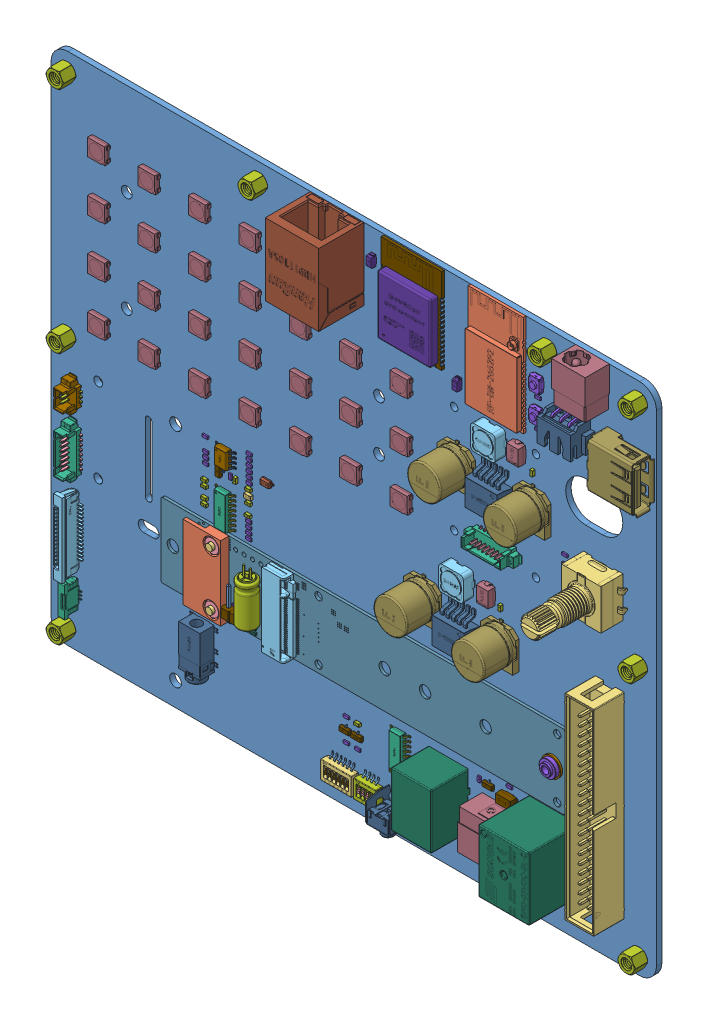
SolidWorks assembly HOUZZkitF1_Tester, configuration 默认. Lengths in mm.
Overall size (180.06 153.05 26.45).
872 component instances, 119 part files, 0 mates.
Components (placement in the parent):
- HOUZZkitF1_Tester.step-1: HOUZZkitF1_Tester.step [默认] at origin size (180.06 153.05 26.45)
  - Board.step-1: Board.step [默认] at origin size (180 153 1.6)
    - Open CASCADE STEP translator 7.5 6.1.1.step-1: Open CASCADE STEP translator 7.5 6.1.1.step [默认] at (0 0 -1.6) size (180 153 1.6)
  - JP4.step-1: JP4.step [默认] at origin size (8.85 58.42 12.17)
    - IDC2.54-40P.step-1: IDC2.54-40P.step [默认] at (77.5 -22.5 0) x (0 1 0) z (0 0 1) size (58.42 8.85 12.17)
      - LOGO__.step-1: LOGO__.step [默认] at (-1.2291 1.1 0.166) x (-1 0 0) z (0 0 -1) size (1.2 1.38 0.01)
      - IDC2.54-40P-0.step-1: IDC2.54-40P-0.step [默认] at origin size (58.42 8.85 12.17)
  - L1.step-1: L1.step [默认] at origin size (7.3 7.3 3.65)
    - CDRH73.step-1: CDRH73.step [默认] at (32.5 36.5 -0.15) x (-1 0 0) z (0 0 1) size (7.3 7.3 3.65)
      - LOGO__-1.step-1: LOGO__-1.step [默认] at (0 0.0189 0.4972) x (-1 0 0) z (0 0 -1) size (0.84 0.97 0.01)
      - CDRH73-2.step-1: CDRH73-2.step [默认] at origin size (7.3 7.3 3.65)
  - C28.step-1: C28.step [默认] at origin size (1.6 0.82 0.82)
    - C 0603.step-1: C 0603.step [默认] at (71 35 -1.6) x (1 0 0) z (0 0 -1) size (1.6 0.82 0.82)
      - LOGO__-3.step-1: LOGO__-3.step [默认] at (0 0.0171 -0.0006) x (-1 0 0) z (0 0 -1) size (0.51 0.59 0)
      - C 0603-4.step-1: C 0603-4.step [默认] at origin size (1.6 0.82 0.82)
  - C26.step-1: C26.step [默认] at origin size (1.6 0.82 0.82)
    - C 0603.step-1: C 0603.step [默认] at (71 16 -1.6) x (1 0 0) z (0 0 -1) size (1.6 0.82 0.82)
      - LOGO__-3.step-1: LOGO__-3.step [默认] at (0 0.0171 -0.0006) x (-1 0 0) z (0 0 -1) size (0.51 0.59 0)
      - C 0603-4.step-1: C 0603-4.step [默认] at origin size (1.6 0.82 0.82)
  - R1.step-1: R1.step [默认] at origin size (1.6 0.8 0.4)
    - R 0603.step-1: R 0603.step [默认] at (63.0001 57.5 0) x (1 0 0) z (0 0 1) size (1.6 0.8 0.4)
      - R 0603-5.step-1: R 0603-5.step [默认] at origin size (1.6 0.8 0.4)
      - LOGO__-6.step-1: LOGO__-6.step [默认] at (0.0001 0.0322 -0.0016) x (-1 0 0) z (0 0 -1) size (0.48 0.55 0)
  - L3.step-1: L3.step [默认] at origin size (7.3 7.3 3.65)
    - CDRH73.step-1: CDRH73.step [默认] at (42 77.5 -0.15) x (-1 0 0) z (0 0 1) size (7.3 7.3 3.65)
      - LOGO__-1.step-1: LOGO__-1.step [默认] at (0 0.0189 0.4972) x (-1 0 0) z (0 0 -1) size (0.84 0.97 0.01)
      - CDRH73-2.step-1: CDRH73-2.step [默认] at origin size (7.3 7.3 3.65)
  - IC5.step-1: IC5.step [默认] at origin size (10 13.33 4.5)
    - TO263-5A.step-1: TO263-5A.step [默认] at (32.5 30 0) x (-1 0 0) z (0 0 1) size (10 13.33 4.5)
  - IC4.step-1: IC4.step [默认] at origin size (10 13.33 4.5)
    - TO263-5A.step-1: TO263-5A.step [默认] at (42.3 70.5 0) x (-1 0 0) z (0 0 1) size (10 13.33 4.5)
  - E7.step-1: E7.step [默认] at origin size (10.3 11.6 10.21)
    - CM F(10X10.2).step-1: CM F(10X10.2).step [默认] at (31 65 0) x (1 0 0) z (0 0 1) size (10.3 11.6 10.21)
      - LOGO__-7.step-1: LOGO__-7.step [默认] at (-0.0044 0.0128 -0.0035) x (-1 0 0) z (0 0 -1) size (1.8 2.08 0.01)
      - CM F(10X10.2)-8.step-1: CM F(10X10.2)-8.step [默认] at origin size (10.3 11.6 10.21)
  - E6.step-1: E6.step [默认] at origin size (10.3 11.6 10.21)
    - CM F(10X10.2).step-1: CM F(10X10.2).step [默认] at (53.5 65 0) x (1 0 0) z (0 0 1) size (10.3 11.6 10.21)
      - LOGO__-7.step-1: LOGO__-7.step [默认] at (-0.0044 0.0128 -0.0035) x (-1 0 0) z (0 0 -1) size (1.8 2.08 0.01)
      - CM F(10X10.2)-8.step-1: CM F(10X10.2)-8.step [默认] at origin size (10.3 11.6 10.21)
  - E5.step-1: E5.step [默认] at origin size (10.3 11.6 10.21)
    - CM F(10X10.2).step-1: CM F(10X10.2).step [默认] at (21 25.5 0) x (1 0 0) z (0 0 1) size (10.3 11.6 10.21)
      - LOGO__-7.step-1: LOGO__-7.step [默认] at (-0.0044 0.0128 -0.0035) x (-1 0 0) z (0 0 -1) size (1.8 2.08 0.01)
      - CM F(10X10.2)-8.step-1: CM F(10X10.2)-8.step [默认] at origin size (10.3 11.6 10.21)
  - E4.step-1: E4.step [默认] at origin size (10.3 11.6 10.21)
    - CM F(10X10.2).step-1: CM F(10X10.2).step [默认] at (44 25.5 0) x (1 0 0) z (0 0 1) size (10.3 11.6 10.21)
      - LOGO__-7.step-1: LOGO__-7.step [默认] at (-0.0044 0.0128 -0.0035) x (-1 0 0) z (0 0 -1) size (1.8 2.08 0.01)
      - CM F(10X10.2)-8.step-1: CM F(10X10.2)-8.step [默认] at origin size (10.3 11.6 10.21)
  - D4.step-1: D4.step [默认] at origin size (3.6 5.31 2.31)
    - SMB.step-1: SMB.step [默认] at (49.5001 77.4771 0.05) x (0 1 0) z (0 0 1) size (5.31 3.6 2.31)
      - SMB-9.step-1: SMB-9.step [默认] at origin size (5.31 3.6 2.3)
      - LOGO__________.____.step-1: LOGO__________.____.step [默认] at (-0.0044 0 -0.003) x (-1 0 0) z (0 0 -1) size (0.9 1.04 0.01)
  - D3.step-1: D3.step [默认] at origin size (3.6 5.31 2.31)
    - SMB.step-1: SMB.step [默认] at (40.5001 36.4771 0.05) x (0 1 0) z (0 0 1) size (5.31 3.6 2.31)
      - SMB-9.step-1: SMB-9.step [默认] at origin size (5.31 3.6 2.3)
      - LOGO__________.____.step-1: LOGO__________.____.step [默认] at (-0.0044 0 -0.003) x (-1 0 0) z (0 0 -1) size (0.9 1.04 0.01)
  - U7.step-1: U7.step [默认] at origin size (10.31 17.9 2.7)
    - SOP28.step-1: SOP28.step [默认] at (62.5 32.5 -1.6) x (1 0 0) z (0 0 -1) size (10.31 17.9 2.7)
      - LOGO__0.5.step-1: LOGO__0.5.step [默认] at (0.0116 0 0.095) x (0 -1 0) z (0 0 -1) size (1.5 1.73 0.01)
      - SOP28 ____.step-1: SOP28 ____.step [默认] at origin size (7.7 17.9 2.6)
      - ________2.6 ____________.step-1: ________2.6 ____________.step [默认] at (3.85 8.26 1.4) x (0 1 0) z (0 0 1) size (0.5 1.3 1.5)
      - ________2.6 ____________.step-2: ________2.6 ____________.step [默认] at (3.85 6.99 1.4) x (0 1 0) z (0 0 1) size (0.5 1.3 1.5)
      - ________2.6 ____________.step-3: ________2.6 ____________.step [默认] at (3.85 5.72 1.4) x (0 1 0) z (0 0 1) size (0.5 1.3 1.5)
      - ________2.6 ____________.step-4: ________2.6 ____________.step [默认] at (3.85 4.45 1.4) x (0 1 0) z (0 0 1) size (0.5 1.3 1.5)
      - ________2.6 ____________.step-5: ________2.6 ____________.step [默认] at (3.85 3.18 1.4) x (0 1 0) z (0 0 1) size (0.5 1.3 1.5)
      - ________2.6 ____________.step-6: ________2.6 ____________.step [默认] at (3.85 1.91 1.4) x (0 1 0) z (0 0 1) size (0.5 1.3 1.5)
      - ________2.6 ____________.step-7: ________2.6 ____________.step [默认] at (3.85 0.64 1.4) x (0 1 0) z (0 0 1) size (0.5 1.3 1.5)
      - ________2.6 ____________.step-8: ________2.6 ____________.step [默认] at (3.85 -0.63 1.4) x (0 1 0) z (0 0 1) size (0.5 1.3 1.5)
      - ________2.6 ____________.step-9: ________2.6 ____________.step [默认] at (3.85 -1.9 1.4) x (0 1 0) z (0 0 1) size (0.5 1.3 1.5)
      - ________2.6 ____________.step-10: ________2.6 ____________.step [默认] at (3.85 -3.17 1.4) x (0 1 0) z (0 0 1) size (0.5 1.3 1.5)
      - ________2.6 ____________.step-11: ________2.6 ____________.step [默认] at (3.85 -4.44 1.4) x (0 1 0) z (0 0 1) size (0.5 1.3 1.5)
      - ________2.6 ____________.step-12: ________2.6 ____________.step [默认] at (3.85 -5.71 1.4) x (0 1 0) z (0 0 1) size (0.5 1.3 1.5)
      - ________2.6 ____________.step-13: ________2.6 ____________.step [默认] at (3.85 -6.98 1.4) x (0 1 0) z (0 0 1) size (0.5 1.3 1.5)
      - ________2.6 ____________.step-14: ________2.6 ____________.step [默认] at (3.85 -8.25 1.4) x (0 1 0) z (0 0 1) size (0.5 1.3 1.5)
      - ________2.6 ____________.step-15: ________2.6 ____________.step [默认] at (-3.85 8.26 1.4) x (0 -1 0) z (0 0 1) size (0.5 1.3 1.5)
      - ________2.6 ____________.step-16: ________2.6 ____________.step [默认] at (-3.85 6.99 1.4) x (0 -1 0) z (0 0 1) size (0.5 1.3 1.5)
      - ________2.6 ____________.step-17: ________2.6 ____________.step [默认] at (-3.85 5.72 1.4) x (0 -1 0) z (0 0 1) size (0.5 1.3 1.5)
      - ________2.6 ____________.step-18: ________2.6 ____________.step [默认] at (-3.85 4.45 1.4) x (0 -1 0) z (0 0 1) size (0.5 1.3 1.5)
      - ________2.6 ____________.step-19: ________2.6 ____________.step [默认] at (-3.85 3.18 1.4) x (0 -1 0) z (0 0 1) size (0.5 1.3 1.5)
      - ________2.6 ____________.step-20: ________2.6 ____________.step [默认] at (-3.85 1.91 1.4) x (0 -1 0) z (0 0 1) size (0.5 1.3 1.5)
      - ________2.6 ____________.step-21: ________2.6 ____________.step [默认] at (-3.85 0.64 1.4) x (0 -1 0) z (0 0 1) size (0.5 1.3 1.5)
      - ________2.6 ____________.step-22: ________2.6 ____________.step [默认] at (-3.85 -0.63 1.4) x (0 -1 0) z (0 0 1) size (0.5 1.3 1.5)
      - ________2.6 ____________.step-23: ________2.6 ____________.step [默认] at (-3.85 -1.9 1.4) x (0 -1 0) z (0 0 1) size (0.5 1.3 1.5)
      - ________2.6 ____________.step-24: ________2.6 ____________.step [默认] at (-3.85 -3.17 1.4) x (0 -1 0) z (0 0 1) size (0.5 1.3 1.5)
      - ________2.6 ____________.step-25: ________2.6 ____________.step [默认] at (-3.85 -4.44 1.4) x (0 -1 0) z (0 0 1) size (0.5 1.3 1.5)
      - ________2.6 ____________.step-26: ________2.6 ____________.step [默认] at (-3.85 -5.71 1.4) x (0 -1 0) z (0 0 1) size (0.5 1.3 1.5)
      - ________2.6 ____________.step-27: ________2.6 ____________.step [默认] at (-3.85 -6.98 1.4) x (0 -1 0) z (0 0 1) size (0.5 1.3 1.5)
      - ________2.6 ____________.step-28: ________2.6 ____________.step [默认] at (-3.85 -8.25 1.4) x (0 -1 0) z (0 0 1) size (0.5 1.3 1.5)
  - U6.step-1: U6.step [默认] at origin size (10.31 17.9 2.7)
    - SOP28.step-1: SOP28.step [默认] at (62.5 13.5 -1.6) x (1 0 0) z (0 0 -1) size (10.31 17.9 2.7)
      - LOGO__0.5.step-1: LOGO__0.5.step [默认] at (0.0116 0 0.095) x (0 -1 0) z (0 0 -1) size (1.5 1.73 0.01)
      - SOP28 ____.step-1: SOP28 ____.step [默认] at origin size (7.7 17.9 2.6)
      - ________2.6 ____________.step-1: ________2.6 ____________.step [默认] at (3.85 8.26 1.4) x (0 1 0) z (0 0 1) size (0.5 1.3 1.5)
      - ________2.6 ____________.step-2: ________2.6 ____________.step [默认] at (3.85 6.99 1.4) x (0 1 0) z (0 0 1) size (0.5 1.3 1.5)
      - ________2.6 ____________.step-3: ________2.6 ____________.step [默认] at (3.85 5.72 1.4) x (0 1 0) z (0 0 1) size (0.5 1.3 1.5)
      - ________2.6 ____________.step-4: ________2.6 ____________.step [默认] at (3.85 4.45 1.4) x (0 1 0) z (0 0 1) size (0.5 1.3 1.5)
      - ________2.6 ____________.step-5: ________2.6 ____________.step [默认] at (3.85 3.18 1.4) x (0 1 0) z (0 0 1) size (0.5 1.3 1.5)
      - ________2.6 ____________.step-6: ________2.6 ____________.step [默认] at (3.85 1.91 1.4) x (0 1 0) z (0 0 1) size (0.5 1.3 1.5)
      - ________2.6 ____________.step-7: ________2.6 ____________.step [默认] at (3.85 0.64 1.4) x (0 1 0) z (0 0 1) size (0.5 1.3 1.5)
      - ________2.6 ____________.step-8: ________2.6 ____________.step [默认] at (3.85 -0.63 1.4) x (0 1 0) z (0 0 1) size (0.5 1.3 1.5)
      - ________2.6 ____________.step-9: ________2.6 ____________.step [默认] at (3.85 -1.9 1.4) x (0 1 0) z (0 0 1) size (0.5 1.3 1.5)
      - ________2.6 ____________.step-10: ________2.6 ____________.step [默认] at (3.85 -3.17 1.4) x (0 1 0) z (0 0 1) size (0.5 1.3 1.5)
      - ________2.6 ____________.step-11: ________2.6 ____________.step [默认] at (3.85 -4.44 1.4) x (0 1 0) z (0 0 1) size (0.5 1.3 1.5)
      - ________2.6 ____________.step-12: ________2.6 ____________.step [默认] at (3.85 -5.71 1.4) x (0 1 0) z (0 0 1) size (0.5 1.3 1.5)
      - ________2.6 ____________.step-13: ________2.6 ____________.step [默认] at (3.85 -6.98 1.4) x (0 1 0) z (0 0 1) size (0.5 1.3 1.5)
      - ________2.6 ____________.step-14: ________2.6 ____________.step [默认] at (3.85 -8.25 1.4) x (0 1 0) z (0 0 1) size (0.5 1.3 1.5)
      - ________2.6 ____________.step-15: ________2.6 ____________.step [默认] at (-3.85 8.26 1.4) x (0 -1 0) z (0 0 1) size (0.5 1.3 1.5)
      - ________2.6 ____________.step-16: ________2.6 ____________.step [默认] at (-3.85 6.99 1.4) x (0 -1 0) z (0 0 1) size (0.5 1.3 1.5)
      - ________2.6 ____________.step-17: ________2.6 ____________.step [默认] at (-3.85 5.72 1.4) x (0 -1 0) z (0 0 1) size (0.5 1.3 1.5)
      - ________2.6 ____________.step-18: ________2.6 ____________.step [默认] at (-3.85 4.45 1.4) x (0 -1 0) z (0 0 1) size (0.5 1.3 1.5)
      - ________2.6 ____________.step-19: ________2.6 ____________.step [默认] at (-3.85 3.18 1.4) x (0 -1 0) z (0 0 1) size (0.5 1.3 1.5)
      - ________2.6 ____________.step-20: ________2.6 ____________.step [默认] at (-3.85 1.91 1.4) x (0 -1 0) z (0 0 1) size (0.5 1.3 1.5)
      - ________2.6 ____________.step-21: ________2.6 ____________.step [默认] at (-3.85 0.64 1.4) x (0 -1 0) z (0 0 1) size (0.5 1.3 1.5)
      - ________2.6 ____________.step-22: ________2.6 ____________.step [默认] at (-3.85 -0.63 1.4) x (0 -1 0) z (0 0 1) size (0.5 1.3 1.5)
      - ________2.6 ____________.step-23: ________2.6 ____________.step [默认] at (-3.85 -1.9 1.4) x (0 -1 0) z (0 0 1) size (0.5 1.3 1.5)
      - ________2.6 ____________.step-24: ________2.6 ____________.step [默认] at (-3.85 -3.17 1.4) x (0 -1 0) z (0 0 1) size (0.5 1.3 1.5)
      - ________2.6 ____________.step-25: ________2.6 ____________.step [默认] at (-3.85 -4.44 1.4) x (0 -1 0) z (0 0 1) size (0.5 1.3 1.5)
      - ________2.6 ____________.step-26: ________2.6 ____________.step [默认] at (-3.85 -5.71 1.4) x (0 -1 0) z (0 0 1) size (0.5 1.3 1.5)
      - ________2.6 ____________.step-27: ________2.6 ____________.step [默认] at (-3.85 -6.98 1.4) x (0 -1 0) z (0 0 1) size (0.5 1.3 1.5)
      - ________2.6 ____________.step-28: ________2.6 ____________.step [默认] at (-3.85 -8.25 1.4) x (0 -1 0) z (0 0 1) size (0.5 1.3 1.5)
  - R51.step-1: R51.step [默认] at origin size (1.6 0.8 0.4)
    - R 0603.step-1: R 0603.step [默认] at (71.0001 36.5 -1.6) x (1 0 0) z (0 0 -1) size (1.6 0.8 0.4)
      - R 0603-5.step-1: R 0603-5.step [默认] at origin size (1.6 0.8 0.4)
      - LOGO__-6.step-1: LOGO__-6.step [默认] at (0.0001 0.0322 -0.0016) x (-1 0 0) z (0 0 -1) size (0.48 0.55 0)
  - R50.step-1: R50.step [默认] at origin size (1.6 0.8 0.4)
    - R 0603.step-1: R 0603.step [默认] at (71.0001 38 -1.6) x (1 0 0) z (0 0 -1) size (1.6 0.8 0.4)
      - R 0603-5.step-1: R 0603-5.step [默认] at origin size (1.6 0.8 0.4)
      - LOGO__-6.step-1: LOGO__-6.step [默认] at (0.0001 0.0322 -0.0016) x (-1 0 0) z (0 0 -1) size (0.48 0.55 0)
  - R49.step-1: R49.step [默认] at origin size (1.6 0.8 0.4)
    - R 0603.step-1: R 0603.step [默认] at (71.0001 39.5 -1.6) x (1 0 0) z (0 0 -1) size (1.6 0.8 0.4)
      - R 0603-5.step-1: R 0603-5.step [默认] at origin size (1.6 0.8 0.4)
      - LOGO__-6.step-1: LOGO__-6.step [默认] at (0.0001 0.0322 -0.0016) x (-1 0 0) z (0 0 -1) size (0.48 0.55 0)
  - R48.step-1: R48.step [默认] at origin size (1.6 0.8 0.4)
    - R 0603.step-1: R 0603.step [默认] at (54.0001 39 -1.6) x (1 0 0) z (0 0 -1) size (1.6 0.8 0.4)
      - R 0603-5.step-1: R 0603-5.step [默认] at origin size (1.6 0.8 0.4)
      - LOGO__-6.step-1: LOGO__-6.step [默认] at (0.0001 0.0322 -0.0016) x (-1 0 0) z (0 0 -1) size (0.48 0.55 0)
  - R47.step-1: R47.step [默认] at origin size (1.6 0.8 0.4)
    - R 0603.step-1: R 0603.step [默认] at (71.0001 17.5 -1.6) x (1 0 0) z (0 0 -1) size (1.6 0.8 0.4)
      - R 0603-5.step-1: R 0603-5.step [默认] at origin size (1.6 0.8 0.4)
      - LOGO__-6.step-1: LOGO__-6.step [默认] at (0.0001 0.0322 -0.0016) x (-1 0 0) z (0 0 -1) size (0.48 0.55 0)
  - R46.step-1: R46.step [默认] at origin size (1.6 0.8 0.4)
    - R 0603.step-1: R 0603.step [默认] at (71.0001 19 -1.6) x (1 0 0) z (0 0 -1) size (1.6 0.8 0.4)
      - R 0603-5.step-1: R 0603-5.step [默认] at origin size (1.6 0.8 0.4)
      - LOGO__-6.step-1: LOGO__-6.step [默认] at (0.0001 0.0322 -0.0016) x (-1 0 0) z (0 0 -1) size (0.48 0.55 0)
  - R45.step-1: R45.step [默认] at origin size (1.6 0.8 0.4)
    - R 0603.step-1: R 0603.step [默认] at (71.0001 20.5 -1.6) x (1 0 0) z (0 0 -1) size (1.6 0.8 0.4)
      - R 0603-5.step-1: R 0603-5.step [默认] at origin size (1.6 0.8 0.4)
      - LOGO__-6.step-1: LOGO__-6.step [默认] at (0.0001 0.0322 -0.0016) x (-1 0 0) z (0 0 -1) size (0.48 0.55 0)
  - R44.step-1: R44.step [默认] at origin size (1.6 0.8 0.4)
    - R 0603.step-1: R 0603.step [默认] at (54.0001 16.4999 -1.6) x (1 0 0) z (0 0 -1) size (1.6 0.8 0.4)
      - R 0603-5.step-1: R 0603-5.step [默认] at origin size (1.6 0.8 0.4)
      - LOGO__-6.step-1: LOGO__-6.step [默认] at (0.0001 0.0322 -0.0016) x (-1 0 0) z (0 0 -1) size (0.48 0.55 0)
  - R43.step-1: R43.step [默认] at origin size (1.6 0.8 0.4)
    - R 0603.step-1: R 0603.step [默认] at (-31.0001 14.5999 0) x (-1 0 0) z (0 0 1) size (1.6 0.8 0.4)
      - R 0603-5.step-1: R 0603-5.step [默认] at origin size (1.6 0.8 0.4)
      - LOGO__-6.step-1: LOGO__-6.step [默认] at (0.0001 0.0322 -0.0016) x (-1 0 0) z (0 0 -1) size (0.48 0.55 0)
  - R42.step-1: R42.step [默认] at origin size (1.6 0.8 0.4)
    - R 0603.step-1: R 0603.step [默认] at (-31.0001 16.0999 0) x (-1 0 0) z (0 0 1) size (1.6 0.8 0.4)
      - R 0603-5.step-1: R 0603-5.step [默认] at origin size (1.6 0.8 0.4)
      - LOGO__-6.step-1: LOGO__-6.step [默认] at (0.0001 0.0322 -0.0016) x (-1 0 0) z (0 0 -1) size (0.48 0.55 0)
  - R41.step-1: R41.step [默认] at origin size (1.6 0.8 0.4)
    - R 0603.step-1: R 0603.step [默认] at (-31.0001 17.5999 0) x (-1 0 0) z (0 0 1) size (1.6 0.8 0.4)
      - R 0603-5.step-1: R 0603-5.step [默认] at origin size (1.6 0.8 0.4)
      - LOGO__-6.step-1: LOGO__-6.step [默认] at (0.0001 0.0322 -0.0016) x (-1 0 0) z (0 0 -1) size (0.48 0.55 0)
  - R40.step-1: R40.step [默认] at origin size (1.6 0.8 0.4)
    - R 0603.step-1: R 0603.step [默认] at (-31.0001 19.0999 0) x (-1 0 0) z (0 0 1) size (1.6 0.8 0.4)
      - R 0603-5.step-1: R 0603-5.step [默认] at origin size (1.6 0.8 0.4)
      - LOGO__-6.step-1: LOGO__-6.step [默认] at (0.0001 0.0322 -0.0016) x (-1 0 0) z (0 0 -1) size (0.48 0.55 0)
  - R39.step-1: R39.step [默认] at origin size (1.6 0.8 0.4)
    - R 0603.step-1: R 0603.step [默认] at (-43.7999 27.6 0) x (1 0 0) z (0 0 1) size (1.6 0.8 0.4)
      - R 0603-5.step-1: R 0603-5.step [默认] at origin size (1.6 0.8 0.4)
      - LOGO__-6.step-1: LOGO__-6.step [默认] at (0.0001 0.0322 -0.0016) x (-1 0 0) z (0 0 -1) size (0.48 0.55 0)
  - R38.step-1: R38.step [默认] at origin size (1.6 0.8 0.4)
    - R 0603.step-1: R 0603.step [默认] at (-30.9001 33.5 0) x (-1 0 0) z (0 0 1) size (1.6 0.8 0.4)
      - R 0603-5.step-1: R 0603-5.step [默认] at origin size (1.6 0.8 0.4)
      - LOGO__-6.step-1: LOGO__-6.step [默认] at (0.0001 0.0322 -0.0016) x (-1 0 0) z (0 0 -1) size (0.48 0.55 0)
  - R37.step-1: R37.step [默认] at origin size (1.6 0.8 0.4)
    - R 0603.step-1: R 0603.step [默认] at (-43.8001 29.0999 0) x (-1 0 0) z (0 0 1) size (1.6 0.8 0.4)
      - R 0603-5.step-1: R 0603-5.step [默认] at origin size (1.6 0.8 0.4)
      - LOGO__-6.step-1: LOGO__-6.step [默认] at (0.0001 0.0322 -0.0016) x (-1 0 0) z (0 0 -1) size (0.48 0.55 0)
  - R36.step-1: R36.step [默认] at origin size (1.6 0.8 0.4)
    - R 0603.step-1: R 0603.step [默认] at (-43.8001 30.5999 0) x (-1 0 0) z (0 0 1) size (1.6 0.8 0.4)
      - R 0603-5.step-1: R 0603-5.step [默认] at origin size (1.6 0.8 0.4)
      - LOGO__-6.step-1: LOGO__-6.step [默认] at (0.0001 0.0322 -0.0016) x (-1 0 0) z (0 0 -1) size (0.48 0.55 0)
  - R35.step-1: R35.step [默认] at origin size (1.6 0.8 0.4)
    - R 0603.step-1: R 0603.step [默认] at (-30.9001 30.5 0) x (-1 0 0) z (0 0 1) size (1.6 0.8 0.4)
      - R 0603-5.step-1: R 0603-5.step [默认] at origin size (1.6 0.8 0.4)
      - LOGO__-6.step-1: LOGO__-6.step [默认] at (0.0001 0.0322 -0.0016) x (-1 0 0) z (0 0 -1) size (0.48 0.55 0)
  - R34.step-1: R34.step [默认] at origin size (1.6 0.8 0.4)
    - R 0603.step-1: R 0603.step [默认] at (-30.9001 35 0) x (-1 0 0) z (0 0 1) size (1.6 0.8 0.4)
      - R 0603-5.step-1: R 0603-5.step [默认] at origin size (1.6 0.8 0.4)
      - LOGO__-6.step-1: LOGO__-6.step [默认] at (0.0001 0.0322 -0.0016) x (-1 0 0) z (0 0 -1) size (0.48 0.55 0)
  - R33.step-1: R33.step [默认] at origin size (1.6 0.8 0.4)
    - R 0603.step-1: R 0603.step [默认] at (-43.8999 34.5001 0) x (1 0 0) z (0 0 1) size (1.6 0.8 0.4)
      - R 0603-5.step-1: R 0603-5.step [默认] at origin size (1.6 0.8 0.4)
      - LOGO__-6.step-1: LOGO__-6.step [默认] at (0.0001 0.0322 -0.0016) x (-1 0 0) z (0 0 -1) size (0.48 0.55 0)
  - R32.step-1: R32.step [默认] at origin size (1.6 0.8 0.4)
    - R 0603.step-1: R 0603.step [默认] at (-30.8999 32.0001 0) x (1 0 0) z (0 0 1) size (1.6 0.8 0.4)
      - R 0603-5.step-1: R 0603-5.step [默认] at origin size (1.6 0.8 0.4)
      - LOGO__-6.step-1: LOGO__-6.step [默认] at (0.0001 0.0322 -0.0016) x (-1 0 0) z (0 0 -1) size (0.48 0.55 0)
  - R31.step-1: R31.step [默认] at origin size (1.6 0.8 0.4)
    - R 0603.step-1: R 0603.step [默认] at (-30.9001 29 0) x (-1 0 0) z (0 0 1) size (1.6 0.8 0.4)
      - R 0603-5.step-1: R 0603-5.step [默认] at origin size (1.6 0.8 0.4)
      - LOGO__-6.step-1: LOGO__-6.step [默认] at (0.0001 0.0322 -0.0016) x (-1 0 0) z (0 0 -1) size (0.48 0.55 0)
  - R30.step-1: R30.step [默认] at origin size (0.8 1.6 0.4)
    - R 0603.step-1: R 0603.step [默认] at (-36.5 27.9001 0) x (0 1 0) z (0 0 1) size (1.6 0.8 0.4)
      - R 0603-5.step-1: R 0603-5.step [默认] at origin size (1.6 0.8 0.4)
      - LOGO__-6.step-1: LOGO__-6.step [默认] at (0.0001 0.0322 -0.0016) x (-1 0 0) z (0 0 -1) size (0.48 0.55 0)
  - R29.step-1: R29.step [默认] at origin size (1.6 0.8 0.4)
    - R 0603.step-1: R 0603.step [默认] at (-30.9001 36.5 0) x (-1 0 0) z (0 0 1) size (1.6 0.8 0.4)
      - R 0603-5.step-1: R 0603-5.step [默认] at origin size (1.6 0.8 0.4)
      - LOGO__-6.step-1: LOGO__-6.step [默认] at (0.0001 0.0322 -0.0016) x (-1 0 0) z (0 0 -1) size (0.48 0.55 0)
  - Q4.step-1: Q4.step [默认] at origin size (2.4 3 1.05)
    - SOT23-3.step-1: SOT23-3.step [默认] at (-39.6 28 0) x (0 -1 0) z (0 0 1) size (3 2.4 1.05)
      - SOT23-3-10.step-1: SOT23-3-10.step [默认] at origin size (3 1.3 1)
      - SOT23-3 ______.step-1: SOT23-3 ______.step [默认] at (0 0.5461 0.475) size (0.4 0.65 0.55)
      - SOT23-3 ______.step-2: SOT23-3 ______.step [默认] at (-0.95 -0.5461 0.475) x (-1 0 0) z (0 0 1) size (0.4 0.65 0.55)
      - SOT23-3 ______.step-3: SOT23-3 ______.step [默认] at (0.95 -0.5461 0.475) x (-1 0 0) z (0 0 1) size (0.4 0.65 0.55)
      - LOGO__0.15.step-1: LOGO__0.15.step [默认] at (0 -0.0163 0.0485) x (-1 0 0) z (0 0 -1) size (0.45 0.52 0)
  - LB2.step-1: LB2.step [默认] at origin size (2.01 1.21 0.91)
    - FB 0805.step-1: FB 0805.step [默认] at (-30.9 25.7 0) x (-1 0 0) z (0 1 0) size (2 0.91 1.2)
      - FB 0805-11.step-1: FB 0805-11.step [默认] at origin size (2 0.91 1.2)
      - LOGO__0.15-12.step-1: LOGO__0.15-12.step [默认] at (-0.0107 -0.0015 -0.0162) x (1 0 0) z (0 1 0) size (0.45 0.52 0)
  - IC3.step-1: IC3.step [默认] at origin size (6.01 10 1.9)
    - SOP16.step-1: SOP16.step [默认] at (-38 19 0) x (1 0 0) z (0 0 1) size (6.01 10 1.9)
      - LOGO__0.25.step-1: LOGO__0.25.step [默认] at (0.0116 0 0.095) x (0 -1 0) z (0 0 -1) size (0.75 0.87 0.01)
      - SOP16 ____.step-1: SOP16 ____.step [默认] at origin size (3.6 10 1.8)
      - ________1.8 ____________.step-1: ________1.8 ____________.step [默认] at (1.8 4.45 1) x (0 1 0) z (0 0 1) size (0.5 1.2 1.1)
      - ________1.8 ____________.step-2: ________1.8 ____________.step [默认] at (1.8 3.18 1) x (0 1 0) z (0 0 1) size (0.5 1.2 1.1)
      - ________1.8 ____________.step-3: ________1.8 ____________.step [默认] at (1.8 1.91 1) x (0 1 0) z (0 0 1) size (0.5 1.2 1.1)
      - ________1.8 ____________.step-4: ________1.8 ____________.step [默认] at (1.8 0.64 1) x (0 1 0) z (0 0 1) size (0.5 1.2 1.1)
      - ________1.8 ____________.step-5: ________1.8 ____________.step [默认] at (1.8 -0.63 1) x (0 1 0) z (0 0 1) size (0.5 1.2 1.1)
      - ________1.8 ____________.step-6: ________1.8 ____________.step [默认] at (1.8 -1.9 1) x (0 1 0) z (0 0 1) size (0.5 1.2 1.1)
      - ________1.8 ____________.step-7: ________1.8 ____________.step [默认] at (1.8 -3.17 1) x (0 1 0) z (0 0 1) size (0.5 1.2 1.1)
      - ________1.8 ____________.step-8: ________1.8 ____________.step [默认] at (1.8 -4.44 1) x (0 1 0) z (0 0 1) size (0.5 1.2 1.1)
      - ________1.8 ____________.step-9: ________1.8 ____________.step [默认] at (-1.8 4.45 1) x (0 -1 0) z (0 0 1) size (0.5 1.2 1.1)
      - ________1.8 ____________.step-10: ________1.8 ____________.step [默认] at (-1.8 3.18 1) x (0 -1 0) z (0 0 1) size (0.5 1.2 1.1)
      - ________1.8 ____________.step-11: ________1.8 ____________.step [默认] at (-1.8 1.91 1) x (0 -1 0) z (0 0 1) size (0.5 1.2 1.1)
      - ________1.8 ____________.step-12: ________1.8 ____________.step [默认] at (-1.8 0.64 1) x (0 -1 0) z (0 0 1) size (0.5 1.2 1.1)
      - ________1.8 ____________.step-13: ________1.8 ____________.step [默认] at (-1.8 -0.63 1) x (0 -1 0) z (0 0 1) size (0.5 1.2 1.1)
      - ________1.8 ____________.step-14: ________1.8 ____________.step [默认] at (-1.8 -1.9 1) x (0 -1 0) z (0 0 1) size (0.5 1.2 1.1)
      - ________1.8 ____________.step-15: ________1.8 ____________.step [默认] at (-1.8 -3.17 1) x (0 -1 0) z (0 0 1) size (0.5 1.2 1.1)
      - ________1.8 ____________.step-16: ________1.8 ____________.step [默认] at (-1.8 -4.44 1) x (0 -1 0) z (0 0 1) size (0.5 1.2 1.1)
  - IC2.step-1: IC2.step [默认] at origin size (6.01 5 1.9)
    - SOP8.step-1: SOP8.step [默认] at (-37.9 32.6 0) size (6.01 5 1.9)
      - LOGO__0.25-13.step-1: LOGO__0.25-13.step [默认] at (0.0116 0 0.095) x (0 -1 0) z (0 0 -1) size (0.75 0.87 0.01)
      - SOP8 ____.step-1: SOP8 ____.step [默认] at origin size (3.6 5 1.8)
      - ________1.8 ____________-14.step-1: ________1.8 ____________-14.step [默认] at (1.8 1.91 1) x (0 1 0) z (0 0 1) size (0.5 1.2 1.1)
      - ________1.8 ____________-14.step-2: ________1.8 ____________-14.step [默认] at (1.8 0.64 1) x (0 1 0) z (0 0 1) size (0.5 1.2 1.1)
      - ________1.8 ____________-14.step-3: ________1.8 ____________-14.step [默认] at (1.8 -0.63 1) x (0 1 0) z (0 0 1) size (0.5 1.2 1.1)
      - ________1.8 ____________-14.step-4: ________1.8 ____________-14.step [默认] at (1.8 -1.9 1) x (0 1 0) z (0 0 1) size (0.5 1.2 1.1)
      - ________1.8 ____________-14.step-5: ________1.8 ____________-14.step [默认] at (-1.8 1.91 1) x (0 -1 0) z (0 0 1) size (0.5 1.2 1.1)
      - ________1.8 ____________-14.step-6: ________1.8 ____________-14.step [默认] at (-1.8 0.64 1) x (0 -1 0) z (0 0 1) size (0.5 1.2 1.1)
      - ________1.8 ____________-14.step-7: ________1.8 ____________-14.step [默认] at (-1.8 -0.63 1) x (0 -1 0) z (0 0 1) size (0.5 1.2 1.1)
      - ________1.8 ____________-14.step-8: ________1.8 ____________-14.step [默认] at (-1.8 -1.9 1) x (0 -1 0) z (0 0 1) size (0.5 1.2 1.1)
  - D2.step-1: D2.step [默认] at origin size (3.7 1.6 1.22)
    - SOD-123.step-1: SOD-123.step [默认] at (-25.5 32 0.05) x (1 0 0) z (0 0 1) size (3.7 1.6 1.22)
      - SOD-123-15.step-1: SOD-123-15.step [默认] at origin size (3.7 1.6 1.22)
      - LOGO__________.____-16.step-1: LOGO__________.____-16.step [默认] at (-0.0155 0.0364 -0.003) x (-1 0 0) z (0 0 -1) size (0.9 1.04 0.01)
  - C29.step-1: C29.step [默认] at origin size (1.6 0.82 0.82)
    - C 0603.step-1: C 0603.step [默认] at (54 37.5 -1.6) x (1 0 0) z (0 0 -1) size (1.6 0.82 0.82)
      - LOGO__-3.step-1: LOGO__-3.step [默认] at (0 0.0171 -0.0006) x (-1 0 0) z (0 0 -1) size (0.51 0.59 0)
      - C 0603-4.step-1: C 0603-4.step [默认] at origin size (1.6 0.82 0.82)
  - C27.step-1: C27.step [默认] at origin size (1.6 0.82 0.82)
    - C 0603.step-1: C 0603.step [默认] at (54 15 -1.6) x (1 0 0) z (0 0 -1) size (1.6 0.82 0.82)
      - LOGO__-3.step-1: LOGO__-3.step [默认] at (0 0.0171 -0.0006) x (-1 0 0) z (0 0 -1) size (0.51 0.59 0)
      - C 0603-4.step-1: C 0603-4.step [默认] at origin size (1.6 0.82 0.82)
  - C25.step-1: C25.step [默认] at origin size (1.6 0.82 0.82)
    - C 0603.step-1: C 0603.step [默认] at (-44 17.1 0) x (-1 0 0) z (0 0 1) size (1.6 0.82 0.82)
      - LOGO__-3.step-1: LOGO__-3.step [默认] at (0 0.0171 -0.0006) x (-1 0 0) z (0 0 -1) size (0.51 0.59 0)
      - C 0603-4.step-1: C 0603-4.step [默认] at origin size (1.6 0.82 0.82)
  - C24.step-1: C24.step [默认] at origin size (1.6 0.82 0.82)
    - C 0603.step-1: C 0603.step [默认] at (-44 18.7 0) x (-1 0 0) z (0 0 1) size (1.6 0.82 0.82)
      - LOGO__-3.step-1: LOGO__-3.step [默认] at (0 0.0171 -0.0006) x (-1 0 0) z (0 0 -1) size (0.51 0.59 0)
      - C 0603-4.step-1: C 0603-4.step [默认] at origin size (1.6 0.82 0.82)
  - C23.step-1: C23.step [默认] at origin size (1.6 0.82 0.82)
    - C 0603.step-1: C 0603.step [默认] at (-44 23.4 0) x (1 0 0) z (0 0 1) size (1.6 0.82 0.82)
      - LOGO__-3.step-1: LOGO__-3.step [默认] at (0 0.0171 -0.0006) x (-1 0 0) z (0 0 -1) size (0.51 0.59 0)
      - C 0603-4.step-1: C 0603-4.step [默认] at origin size (1.6 0.82 0.82)
  - C22.step-1: C22.step [默认] at origin size (1.6 0.82 0.82)
    - C 0603.step-1: C 0603.step [默认] at (-44 21.8 0) x (-1 0 0) z (0 0 1) size (1.6 0.82 0.82)
      - LOGO__-3.step-1: LOGO__-3.step [默认] at (0 0.0171 -0.0006) x (-1 0 0) z (0 0 -1) size (0.51 0.59 0)
      - C 0603-4.step-1: C 0603-4.step [默认] at origin size (1.6 0.82 0.82)
  - C21.step-1: C21.step [默认] at origin size (1.6 0.82 0.82)
    - C 0603.step-1: C 0603.step [默认] at (-31 20.7 0) x (-1 0 0) z (0 0 1) size (1.6 0.82 0.82)
      - LOGO__-3.step-1: LOGO__-3.step [默认] at (0 0.0171 -0.0006) x (-1 0 0) z (0 0 -1) size (0.51 0.59 0)
      - C 0603-4.step-1: C 0603-4.step [默认] at origin size (1.6 0.82 0.82)
  - C20.step-1: C20.step [默认] at origin size (1.6 0.82 0.82)
    - C 0603.step-1: C 0603.step [默认] at (-30.9 23.9 0) x (-1 0 0) z (0 0 1) size (1.6 0.82 0.82)
      - LOGO__-3.step-1: LOGO__-3.step [默认] at (0 0.0171 -0.0006) x (-1 0 0) z (0 0 -1) size (0.51 0.59 0)
      - C 0603-4.step-1: C 0603-4.step [默认] at origin size (1.6 0.82 0.82)
  - C19.step-1: C19.step [默认] at origin size (1.6 0.82 0.82)
    - C 0603.step-1: C 0603.step [默认] at (-30.9 27.5 0) x (1 0 0) z (0 0 1) size (1.6 0.82 0.82)
      - LOGO__-3.step-1: LOGO__-3.step [默认] at (0 0.0171 -0.0006) x (-1 0 0) z (0 0 -1) size (0.51 0.59 0)
      - C 0603-4.step-1: C 0603-4.step [默认] at origin size (1.6 0.82 0.82)
  - C18.step-1: C18.step [默认] at origin size (0.82 1.6 0.82)
    - C 0603.step-1: C 0603.step [默认] at (-34.8 27.9 0) x (0 1 0) z (0 0 1) size (1.6 0.82 0.82)
      - LOGO__-3.step-1: LOGO__-3.step [默认] at (0 0.0171 -0.0006) x (-1 0 0) z (0 0 -1) size (0.51 0.59 0)
      - C 0603-4.step-1: C 0603-4.step [默认] at origin size (1.6 0.82 0.82)
  - X1.step-1: X1.step [默认] at origin size (2.5 3.2 0.72)
    - OSC 3225-4.step-1: OSC 3225-4.step [默认] at (-18.8196 75.7828 -1.6) x (0 1 0) z (0 0 -1) size (3.2 2.5 0.72)
      - OSC 3225-4-17.step-1: OSC 3225-4-17.step [默认] at origin size (3.2 2.5 0.72)
      - LOGO__0.15-18.step-1: LOGO__0.15-18.step [默认] at (-0.0166 0.0115 -0.003) size (0.45 0.52 0)
  - U5.step-1: U5.step [默认] at origin size (9.01 9.01 1.45)
    - LQFP48-7x7.step-1: LQFP48-7x7.step [默认] at (-10.2343 78.2414 -1.6) x (0 -1 0) z (0 0 -1) size (9.01 9.01 1.45)
      - LQFP48 7x7  ____.step-1: LQFP48 7x7  ____.step [默认] at origin size (7 7 1.4)
      - ______0.25.step-1: ______0.25.step [默认] at (2.75 -3.5 0.75) x (-1 0 0) z (0 0 1) size (0.25 1 0.8)
      - ______0.25.step-2: ______0.25.step [默认] at (2.25 -3.5 0.75) x (-1 0 0) z (0 0 1) size (0.25 1 0.8)
      - ______0.25.step-3: ______0.25.step [默认] at (1.75 -3.5 0.75) x (-1 0 0) z (0 0 1) size (0.25 1 0.8)
      - ______0.25.step-4: ______0.25.step [默认] at (1.25 -3.5 0.75) x (-1 0 0) z (0 0 1) size (0.25 1 0.8)
      - ______0.25.step-5: ______0.25.step [默认] at (0.75 -3.5 0.75) x (-1 0 0) z (0 0 1) size (0.25 1 0.8)
      - ______0.25.step-6: ______0.25.step [默认] at (0.25 -3.5 0.75) x (-1 0 0) z (0 0 1) size (0.25 1 0.8)
      - ______0.25.step-7: ______0.25.step [默认] at (-0.25 -3.5 0.75) x (-1 0 0) z (0 0 1) size (0.25 1 0.8)
      - ______0.25.step-8: ______0.25.step [默认] at (-0.75 -3.5 0.75) x (-1 0 0) z (0 0 1) size (0.25 1 0.8)
      - ______0.25.step-9: ______0.25.step [默认] at (-1.25 -3.5 0.75) x (-1 0 0) z (0 0 1) size (0.25 1 0.8)
      - ______0.25.step-10: ______0.25.step [默认] at (-1.75 -3.5 0.75) x (-1 0 0) z (0 0 1) size (0.25 1 0.8)
      - ______0.25.step-11: ______0.25.step [默认] at (-2.25 -3.5 0.75) x (-1 0 0) z (0 0 1) size (0.25 1 0.8)
      - ______0.25.step-12: ______0.25.step [默认] at (-2.75 -3.5 0.75) x (-1 0 0) z (0 0 1) size (0.25 1 0.8)
      - ______0.25.step-13: ______0.25.step [默认] at (3.5 2.75 0.75) x (0 -1 0) z (0 0 1) size (0.25 1 0.8)
      - ______0.25.step-14: ______0.25.step [默认] at (-2.75 3.5 0.75) size (0.25 1 0.8)
      - ______0.25.step-15: ______0.25.step [默认] at (-3.5 -2.75 0.75) x (0 1 0) z (0 0 1) size (0.25 1 0.8)
      - ______0.25.step-16: ______0.25.step [默认] at (3.5 2.25 0.75) x (0 -1 0) z (0 0 1) size (0.25 1 0.8)
      - ______0.25.step-17: ______0.25.step [默认] at (-2.25 3.5 0.75) size (0.25 1 0.8)
      - ______0.25.step-18: ______0.25.step [默认] at (-3.5 -2.25 0.75) x (0 1 0) z (0 0 1) size (0.25 1 0.8)
      - ______0.25.step-19: ______0.25.step [默认] at (3.5 1.75 0.75) x (0 -1 0) z (0 0 1) size (0.25 1 0.8)
      - ______0.25.step-20: ______0.25.step [默认] at (-1.75 3.5 0.75) size (0.25 1 0.8)
      - ______0.25.step-21: ______0.25.step [默认] at (-3.5 -1.75 0.75) x (0 1 0) z (0 0 1) size (0.25 1 0.8)
      - ______0.25.step-22: ______0.25.step [默认] at (3.5 1.25 0.75) x (0 -1 0) z (0 0 1) size (0.25 1 0.8)
      - ______0.25.step-23: ______0.25.step [默认] at (-1.25 3.5 0.75) size (0.25 1 0.8)
      - ______0.25.step-24: ______0.25.step [默认] at (-3.5 -1.25 0.75) x (0 1 0) z (0 0 1) size (0.25 1 0.8)
      - ______0.25.step-25: ______0.25.step [默认] at (3.5 0.75 0.75) x (0 -1 0) z (0 0 1) size (0.25 1 0.8)
      - ______0.25.step-26: ______0.25.step [默认] at (-0.75 3.5 0.75) size (0.25 1 0.8)
